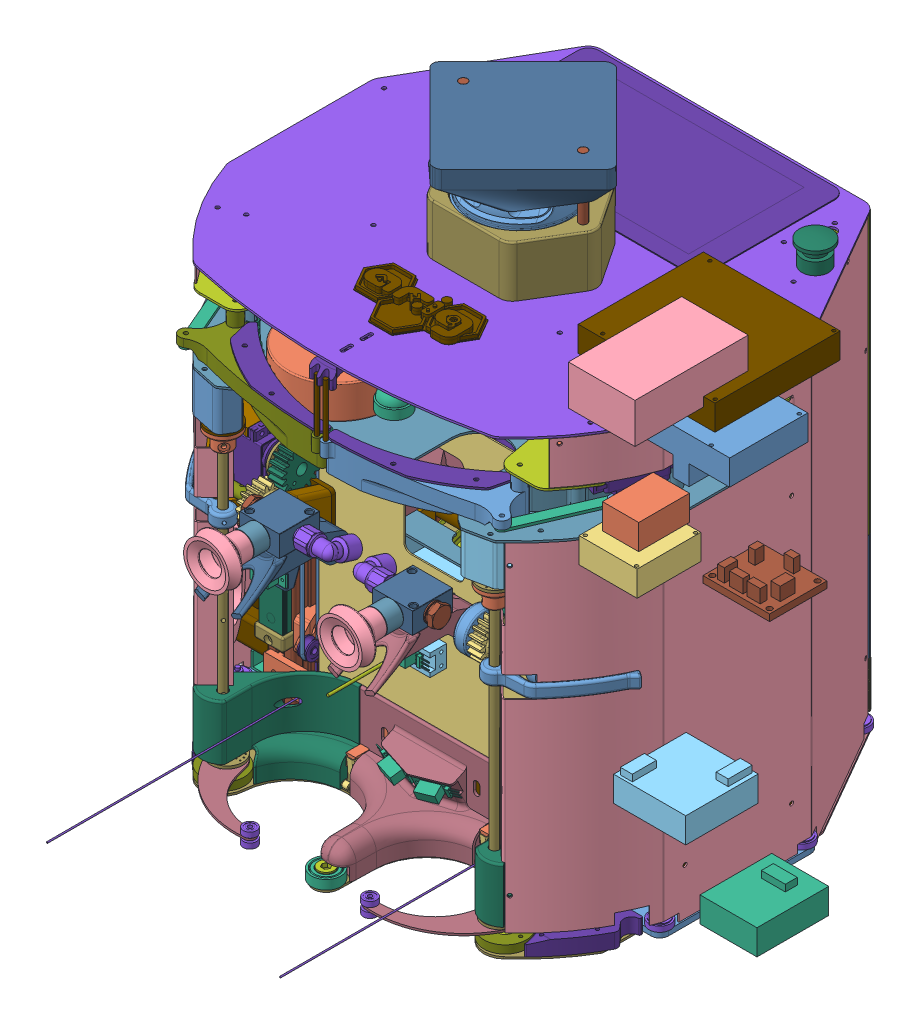
SolidWorks assembly 2019_Gros_robot, configuration Défaut. Lengths in mm. (continued)
Mates (geometry in assembly coordinates): (continued)
- Coaxiale36: concentric anti-aligned: cylinder of roulement-1 through (0 11.5 145.4518) axis (0 1 0) radius 4; cylinder of 20190123-2208-1 through (0 8.1 145.4518) axis (0 -1 0) radius 3.925
- Coïncidente121: coincident anti-aligned: plane of roulement-1 through (2.7957 15 140.7153) normal (0 1 0); plane of 20190123-2208-1 through (5.925 15 145.4518) normal (0 -1 0)
- Coaxiale37: concentric anti-aligned: cylinder of 20190208-2148-1 through (102 235.4 120.9526) axis (0 -1 0) radius 3; cylinder of 20190212-2200-1 through (102 57 120.9526) axis (0 1 0) radius 3.5
- Distance73: distance = 0.8 mm anti-aligned: plane of Roulement_d3xd10xe4-1 through (47.1943 17.95 156.201) normal (0 1 0); plane of 20190208-2207-1 through (102.5 18.75 117.5) normal (0 -1 0)
- Coaxiale39: concentric aligned: cylinder of Roulement_d3xd10xe4-1 through (45.0929 13.95 157.5553) axis (0 -1 0) radius 5; cylinder of 20190208-2207-1 through (45.0929 20.25 157.5553) axis (0 -1 0) radius 1.2
- Tangent1: tangent anti-aligned: cylinder of ? through (50 154.25 120) axis (0 -1 0) radius 38.1; cylinder of Roulement_d3xd10xe4-1 through (49.3866 13.95 163.0956) axis (0 -1 0) radius 5
- Coaxiale42: concentric aligned: cylinder of Roulement_d3xd10xe4-1 through (45.0929 13.95 157.5553) axis (0 -1 0) radius 5; cylinder of Roulement_d3xd10xe4-2 through (45.0929 21.05 157.5553) axis (0 -1 0) radius 5
- Distance74: distance = 0.8 mm anti-aligned: plane of Roulement_d3xd10xe4-2 through (42.6851 21.05 156.8828) normal (0 -1 0); plane of 20190208-2207-1 through (102.5 20.25 117.5) normal (0 1 0)
- Distance80: distance = 50 mm aligned: plane of Palet-1 through (-50 12.7 119.5978) normal (1 0 0); plane of assembly through (0 0 0) normal (1 0 0)
- Coïncidente140: coincident anti-aligned: plane of Robot2019_plaque bille porteuseAvant-1 through (0 7 0) normal (0 1 0); plane of 20190212-2200-1 through (-89.8589 7 116.7694) normal (0 -1 0)
- Coaxiale53: concentric: cylinder of Robot2019_plaque bille porteuseAvant-1 through (-50 7 120) axis (0 -1 0) radius 40; point of 20190212-2200-1
- Parallèle6: parallel anti-aligned: plane of Robot2017_BaseRoulante-1/Robot2015_BaseRoulante_piece01-1 through (0 11 60) normal (0 0 1); plane of 20190212-2200-1 through (-96 29 65) normal (0 0 -1)
- Coïncidente143: coincident anti-aligned: plane of microswitchGaletAss-1/microswitchGalet02-1 through (53.5 29 66) normal (1 0 0); plane of 20190212-2200-1 through (53.5 6.95 144) normal (-1 0 0)
- Coaxiale54: concentric anti-aligned: cylinder of microswitchGaletAss-1/microswitchGalet02-1 through (46.5 14.5 69) axis (1 0 0) radius 1; cylinder of 20190212-2200-1 through (68.5 14.5 69) axis (-1 0 0) radius 1.2
- Coaxiale55: concentric anti-aligned: cylinder of microswitchGaletAss-1/microswitchGalet02-1 through (46.5 23.5 69) axis (1 0 0) radius 1; cylinder of 20190212-2200-1 through (68.5 23.5 69) axis (-1 0 0) radius 1.2
- Coaxiale56: concentric aligned: cylinder of BillePorteuse2019-1 through (105.917 10 116.9526) axis (0 1 0) radius 6.4; cylinder of 20190214-0012-1 through (105.917 4.7 116.9526) axis (0 1 0) radius 8
- Coïncidente144: coincident anti-aligned: plane of BillePorteuse2019-1 through (110.9612 4.7 110.7432) normal (0 1 0); plane of 20190214-0012-1 through (105.917 4.7 116.9526) normal (0 -1 0)
- Coïncidente147: coincident anti-aligned: circle of Servo_HS-85-BB-1; circle of Access_HS-645_BrasRondPetitModele-1
- Coaxiale57: concentric anti-aligned: cylinder of 20190208-2207-1 through (102.5 20.25 117.5) axis (0 -1 0) radius 12; cylinder of Access_HS-645_BrasRondPetitModele-1 through (102.5 24.75 117.5) axis (0 1 0) radius 12
- Coïncidente148: coincident anti-aligned: plane of 20190208-2207-1 through (102.5 20.25 117.5) normal (0 1 0); plane of Access_HS-645_BrasRondPetitModele-1 through (100.0867 20.25 120.3703) normal (0 -1 0)
- Coaxiale58: concentric anti-aligned: cylinder of 20190208-2207-1 through (105.415 18.75 109.5155) axis (0 1 0) radius 1.2; cylinder of Access_HS-645_BrasRondPetitModele-1 through (105.415 30.25 109.5155) axis (0 -1 0) radius 0.5
- Coaxiale59: concentric aligned: cylinder of 20190208-2207-1 through (102.5 20.25 117.5) axis (0 -1 0) radius 12; cylinder of 20190208-2207-2 through (102.5 20.25 117.5) axis (0 -1 0) radius 12
- Angle2: planar angle = 3.185226 rad aligned: plane of 20190208-2207-1 through (102.5 18.75 117.5) normal (-0.572218 0 -0.820101); plane of 20190208-2207-2 through (102.5 18.75 117.5) normal (0.607446 0 0.794361)
- Distance82: distance = 96 mm anti-aligned: plane of Servo_HS-85-BB-1 through (96 25.85 124) normal (-1 0 0); plane of assembly through (0 0 0) normal (1 0 0)
- Distance83: distance = 117.5 mm: point of 20190208-2207-1; plane of assembly
- Distance84: distance = 30 mm aligned: plane of Servo_HS-85-BB-1 through (102.5 37 117.5) normal (0 1 0); plane of Robot2019_plaque bille porteuseAvant-1 through (0 7 0) normal (0 1 0)
- Coaxiale61: concentric aligned: cylinder of Robot2019_plaque bille porteuseAvant-1 through (105.917 7 116.9526) axis (0 -1 0) radius 16; cylinder of 20190214-0012-1 through (105.917 14.7 116.9526) axis (0 -1 0) radius 16
- Coïncidente151: coincident aligned: plane of 20190208-2207-1 through (102.5 20.25 117.5) normal (0 1 0); plane of 20190208-2207-2 through (102.5 20.25 117.5) normal (0 1 0)
- Coaxiale62: concentric aligned: cylinder of Robot2019_plaque bille porteuseAvant-1 through (100.1435 7 126.9526) axis (0 -1 0) radius 1.5; cylinder of 20190214-0012-1 through (100.1435 14.7 126.9526) axis (0 -1 0) radius 1.2
- Coaxiale63: concentric aligned: cylinder of 20181001-2148-1 through (-7.4687 58.1355 42.4725) axis (0.258819 -0.408218 0.875426) radius 0.65; cylinder of 20170416-2304-1/pololu gp2y0d805-1 through (3.2601 41.2137 78.7615) axis (0.258819 -0.408218 0.875426) radius 1
- Coïncidente152: coincident anti-aligned: plane of 20181001-2148-1 through (0 51.0665 85.3479) normal (0.258819 -0.408218 0.875426); plane of 20170416-2304-1/pololu gp2y0d805-1 through (1.0782 36.4945 78.234) normal (-0.258819 0.408218 -0.875426)
- Parallèle7: parallel aligned: plane of 20181001-2148-1 through (1.0353 36.8864 76.4144) normal (0 0.906308 0.422618); plane of 20170416-2304-1/pololu gp2y0d805-1 through (1.4924 43.9981 83.4383) normal (0 0.906308 0.422618)
- Coïncidente157: coincident anti-aligned: plane of Robot2019_plaque bille porteuseAvant-1 through (0 7 0) normal (0 1 0); plane of 20190219-0006-1 through (105.917 7 116.9526) normal (0 -1 0)
- Coaxiale64: concentric aligned: cylinder of Robot2019_plaque bille porteuseAvant-1 through (0 7 0) axis (0 -1 0) radius 173.7857; cylinder of 20190219-0006-1 through (0 18 0) axis (0 -1 0) radius 174
- Coïncidente158: coincident aligned: plane of 20190219-0006-1 through (0 7 0) normal (0 0 1); plane of assembly through (0 0 0) normal (0 0 1)
- Coïncidente159: coincident aligned: plane of Roulement_d3xd10xe4-1 through (47.1943 13.95 156.201) normal (0 -1 0); plane of Roulement_d3xd10xe4-3 through (160.2067 13.95 73.6245) normal (0 -1 0)
- Coaxiale65: concentric aligned: cylinder of 20190208-2207-2 through (158.1053 20.25 74.9788) axis (0 -1 0) radius 4; cylinder of Roulement_d3xd10xe4-3 through (158.1053 13.95 74.9788) axis (0 -1 0) radius 5
- Coïncidente161: coincident anti-aligned: plane of 20190219-0101-1 through (130 61.0678 59) normal (-1 0 0); plane of Robot2019_profiléX20_02-3 through (130 11 46.7) normal (1 0 0)
- Distance86: distance = 1 mm aligned: plane of 20190219-0101-1 through (130 61.0678 59) normal (0 0 1); plane of Robot2019_profiléX20_02-3 through (123.3 11 60) normal (0 0 1)
- Coïncidente162: coincident aligned: plane of 20190219-0101-1 through (163 14.6933 37) normal (1 0 0); plane of 20190219-0101-2 through (163 87.4423 -37) normal (1 0 0)
- Coïncidente163: coincident aligned: plane of 20190219-0101-1 through (130 61.0678 50) normal (0 1 0); plane of 20190219-0101-2 through (130 61.0678 -50) normal (0 1 0)
- Distance87: distance = 1 mm aligned: plane of 20190219-0101-2 through (130 41.0678 -59) normal (0 0 -1); plane of Robot2019_profiléX20_02-4 through (128 11 -60) normal (0 0 -1)
- Coaxiale66: concentric aligned: cylinder of 20190208-2148-1 through (102 235.4 120.9526) axis (0 -1 0) radius 3; cylinder of 20190220-2148-1 through (102 186.4 120.9526) axis (0 -1 0) radius 3.1
- Coaxiale67: concentric aligned: cylinder of Servo_HS-85-BB-2 through (102 241.9 120.9526) axis (0 1 0) radius 2.75; cylinder of Access_HS-645_BrasRondPetitModele-2 through (102 244.9 120.9526) axis (0 1 0) radius 2.75
- Coïncidente164: coincident anti-aligned: plane of Servo_HS-85-BB-2 through (102 241.9 120.9526) normal (0 -1 0); plane of Access_HS-645_BrasRondPetitModele-2 through (99.4128 241.9 121.8847) normal (0 1 0)
- Coïncidente165: coincident anti-aligned: plane of Robot2019_plaque du dessus-1 through (0 276 -355) normal (0 -1 0); plane of Servo_HS-85-BB-2 through (102 276 120.9526) normal (0 1 0)
- Coaxiale68: concentric anti-aligned: cylinder of 20190208-2148-1 through (102 235.4 120.9526) axis (0 -1 0) radius 3; cylinder of Access_HS-645_BrasRondPetitModele-2 through (102 244.9 120.9526) axis (0 1 0) radius 12
- Coaxiale70: concentric aligned: cylinder of Access_HS-645_BrasRondPetitModele-2 through (102 244.9 120.9526) axis (0 1 0) radius 12; cylinder of 20190221-0033-1 through (102 240.4 120.9526) axis (0 1 0) radius 12
- Coïncidente168: coincident anti-aligned: plane of Access_HS-645_BrasRondPetitModele-2 through (98.472 240.4 122.2237) normal (0 -1 0); plane of 20190221-0033-1 through (99.4389 240.4 117.88) normal (0 1 0)
- Coaxiale71: concentric anti-aligned: cylinder of Access_HS-645_BrasRondPetitModele-2 through (95.5972 250.4 113.2712) axis (0 -1 0) radius 0.5; cylinder of 20190221-0033-1 through (95.5972 225.4 113.2712) axis (0 1 0) radius 1.2
- Distance91: distance = 4 mm aligned: plane of Raspberry pi3 Screen assembly-1 through (-9.296 346 -101.85) normal (0 1 0); plane of assembly through (0 350 0) normal (0 1 0)
- Coaxiale72: concentric aligned: cylinder of 20190208-2148-1 through (99.6956 229.4 122.8734) axis (0.768138 0 -0.640285) radius 1.25; cylinder of 20190221-0033-1 through (92.7823 229.4 128.636) axis (0.768138 0 -0.640285) radius 1.5
- Coaxiale73: concentric aligned: cylinder of 20190208-2148-1 through (99.6956 181.4 122.8734) axis (0.768138 0 -0.640285) radius 1.25; cylinder of 20190220-2148-1 through (108.1451 181.4 115.8303) axis (0.768138 0 -0.640285) radius 1.2
- AngleLimite1: limit planar angle = 0.418879 rad aligned: plane of 20190220-2148-1 through (102 181.4 120.9526) normal (0.913545 0 0.406737); plane of assembly through (0 0 0) normal (1 0 0)
- Coïncidente169: coincident aligned: plane of Carter2019-1 through (0 7 0) normal (0 0 1); plane of assembly through (0 0 0) normal (0 0 1)
- Coïncidente170: coincident aligned: plane of Carter2019-1 through (0 7 0) normal (1 0 0); plane of assembly through (0 0 0) normal (1 0 0)
- Coïncidente171: coincident anti-aligned: plane of Robot2017_BaseRoulante-1/Robot2015_BaseRoulante_piece01-1 through (0 7 0) normal (0 -1 0); plane of Carter2019-1 through (0 7 0) normal (0 1 0)
- Coïncidente172: coincident anti-aligned: plane of Robot2019_plaque du dessus-1 through (0 276 -355) normal (0 -1 0); plane of 20190223-1730-1 through (-0.1299 276 -354.8724) normal (0 1 0)
- Coïncidente173: coincident anti-aligned: plane of Servo_HS-85-BB-2 through (124.7356 246 115.3317) normal (0.5 0 0.866025); plane of 20190223-1730-1 through (125.0387 276 115.1567) normal (-0.5 0 -0.866025)
- Coaxiale75: concentric aligned: cylinder of Servo_HS-85-BB-2 through (93.6429 257.15 125.7776) axis (0 -1 0) radius 1.5; cylinder of 20190223-1730-1 through (93.6429 276 125.7776) axis (0 -1 0) radius 1.2
- Parallèle9: parallel aligned: plane of assembly through (0 0 0) normal (1 0 0); plane of 20190223-1730-1 through (-0.1299 256 0.1276) normal (1 0 0)
- Coaxiale76: concentric aligned: cylinder of 20181002-0030-1/20181002-0031-4 through (0 293.5 0) axis (0 -1 0) radius 141; cylinder of 20181002-0216-1/20181002-0217-1 through (0 296.5 0) axis (0 -1 0) radius 141
- Coïncidente175: coincident anti-aligned: plane of 20181001-2148-1 through (0 51.0665 85.3479) normal (-0.258819 -0.408218 0.875426); plane of 20170416-2304-2/pololu gp2y0d805-1 through (-1.0782 44.6512 82.0376) normal (0.258819 0.408218 -0.875426)
- Coaxiale77: concentric aligned: cylinder of 20181001-2148-1 through (7.4687 58.1355 42.4725) axis (-0.258819 -0.408218 0.875426) radius 0.65; cylinder of 20170416-2304-2/pololu gp2y0d805-1 through (-3.2601 41.2137 78.7615) axis (-0.258819 -0.408218 0.875426) radius 1
- Parallèle10: parallel aligned: plane of 20181001-2148-1 through (1.0353 36.8864 76.4144) normal (0 0.906308 0.422618); plane of 20170416-2304-2/pololu gp2y0d805-1 through (-1.4924 43.9981 83.4383) normal (0 0.906308 0.422618)
- Coaxiale78: concentric aligned: cylinder of Robot2019_plaque du dessus-1 through (0 267.5 0) axis (0 1 0) radius 27; cylinder of 20190221-0152-1 through (0 274.2 0) axis (0 1 0) radius 25.3
- Distance94: distance = 1.5 mm anti-aligned: plane of 20190221-0152-1 through (0 311 0) normal (0 -1 0); plane of 20181002-0030-1/20181002-0031-2 through (0 309.5 0) normal (0 1 0)
- Coïncidente177: coincident anti-aligned: plane of 20190221-0152-1; plane of assembly through (0 0 0) normal (1 0 0)
- Coïncidente178: coincident anti-aligned: plane of Symétrie20181002-0216-3/Symétrie20181002-0217-1 through (114.2513 290.5 136.5049) normal (0 -1 0); plane of 20190225-2214-1 through (118.6064 290.5 132.1497) normal (0 1 0)
- Coaxiale79: concentric aligned: cylinder of Symétrie20181002-0216-3/Symétrie20181002-0217-1 through (118.6064 430.1481 132.1497) axis (0 -1 0) radius 1.5; cylinder of 20190225-2214-1 through (118.6064 290.5 132.1497) axis (0 -1 0) radius 1.5
- Coaxiale80: concentric anti-aligned: cylinder of Access_HS-485_BrasReglablePartieB-1 through (143.565 290.05 74.3045) axis (0 1 0) radius 0.5; cylinder of 20190225-2214-1 through (143.565 290.5 74.3045) axis (0 -1 0) radius 1.5
- Coïncidente179: coincident anti-aligned: plane of 20181002-0030-1/20181002-0031-2 through (0 309.5 0) normal (0 1 0); plane of Robot2019_plaque elec-1 through (0 309.5 -355) normal (0 -1 0)
- Coaxiale83: concentric anti-aligned: cylinder of Robot2019_plaque elec-1 through (143 301 86.913) axis (0 1 0) radius 1.5; cylinder of Servo_HS-485-HB-1 through (143 309.5 86.913) axis (0 -1 0) radius 1.5
- Parallèle13: parallel aligned: plane of Servo_HS-485-HB-1 through (159.9911 312.35 48.1691) normal (0.95652 0 0.291667); plane of Robot2019_plaque elec-1 through (141.4855 301 40.4511) normal (0.95652 0 0.291667)
- AngleLimite2: limit planar angle = 0 rad anti-aligned: plane of Robot2019_plaque du dessus-1 through (30 275.999 141.0123) normal (0.130526 0 0.991445); plane of Symétrie20181002-0216-3/Symétrie20181002-0217-1 through (0.3812 243.6998 144.987) normal (-0.130526 0 -0.991445)
- Distance95: distance = 5 mm aligned: plane of Robot2019_plaque superieure-2 through (0 345 -355) normal (0 1 0); plane of assembly through (0 350 0) normal (0 1 0)
- Coïncidente185: coincident anti-aligned: plane of rplidar-a2-1 through (0 362.5 0) normal (0 -1 0); plane of 20161105-0900-1 through (0 362.5 0) normal (0 1 0)
- Coaxiale85: concentric anti-aligned: cylinder of rplidar-a2-1 through (-20.8597 362.5 20.8597) axis (0 1 0) radius 1.6; cylinder of 20161105-0900-1 through (-20.8597 380.5 20.8597) axis (0 -1 0) radius 1.5
- Coaxiale86: concentric anti-aligned: cylinder of rplidar-a2-1 through (-20.8597 362.5 -20.8597) axis (0 1 0) radius 1.6; cylinder of 20161105-0900-1 through (-20.8597 380.5 -20.8597) axis (0 -1 0) radius 1.5
- Coaxiale87: concentric aligned: cylinder of 20161105-0900-1 through (-45 380.5 -2.5) axis (0 -1 0) radius 3; cylinder of 20161106-1538-1 through (-45 430 -2.5) axis (0 -1 0) radius 3
- Coaxiale88: concentric aligned: cylinder of 20190313-2117-1 through (-45 430 -2.5) axis (0 -1 0) radius 3.1; cylinder of 20161106-1538-1 through (-45 430 -2.5) axis (0 -1 0) radius 3
- Coaxiale89: concentric aligned: cylinder of 20161105-0900-1 through (45 380.5 -2.5) axis (0 -1 0) radius 3; cylinder of 20161106-1538-2 through (45 430 -2.5) axis (0 -1 0) radius 3
- Coaxiale90: concentric aligned: cylinder of 20190313-2117-1 through (45 430 -2.5) axis (0 -1 0) radius 3.1; cylinder of 20161106-1538-2 through (45 430 -2.5) axis (0 -1 0) radius 3
- Coïncidente186: coincident aligned: plane of 20190313-2117-1 through (0 430 -2.5) normal (0 1 0); plane of 20161106-1538-2 through (45 430 -2.5) normal (0 1 0)
- Coïncidente187: coincident aligned: plane of 20190313-2117-1 through (0 430 -2.5) normal (0 1 0); plane of 20161106-1538-1 through (-45 430 -2.5) normal (0 1 0)
- Coïncidente188: coincident anti-aligned: plane of Robot2019_plaque superieure-2 through (0 345 -355) normal (0 1 0); plane of 20161105-0900-1 through (45 345 -2.5) normal (0 -1 0)
- Coïncidente189: coincident aligned: plane of 20190313-2117-1 through (0 430 -2.5) normal (0 1 0); plane of assembly through (0 430 0) normal (0 1 0)
- Coïncidente190: coincident aligned: plane of 20161105-0900-1 through (0 345 0) normal (0 0 1); plane of assembly through (0 0 0) normal (0 0 1)
- Coïncidente191: coincident aligned: plane of 20161105-0900-1 through (0 345 0) normal (1 0 0); plane of assembly through (0 0 0) normal (1 0 0)
- Distance96: distance = 1 mm anti-aligned: plane of Robot2019_plaque superieure-2 through (76.184 342 -152) normal (-1 0 0); plane of Raspberry pi3 Screen assembly-1 through (75.184 340.04 -50) normal (1 0 0)
- Distance97: distance = 2 mm aligned: plane of 20170416-2304-3/SupportCapteurPololu-1 through (-128 238.5 -30) normal (-1 0 0); plane of Robot2019_profiléX20_02-2 through (-130 11 -46.7) normal (-1 0 0)
- Distance98: distance = 40 mm aligned: plane of 20170416-2304-3/SupportCapteurPololu-1 through (-120 226 0) normal (0 0 1); plane of Robot2019_profiléX20_02-2 through (-128 11 -40) normal (0 0 1)
- Distance99: distance = 50 mm aligned: plane of 20170416-2304-3/SupportCapteurPololu-1 through (-128 226 -30) normal (0 -1 0); plane of Robot2019_plaque du dessus-1 through (0 276 -355) normal (0 -1 0)
- Distance100: distance = 3 mm anti-aligned: plane of Adafruit_TCS34725-1 through (-106.6 273 31) normal (0 1 0); plane of Robot2019_plaque du dessus-1 through (0 276 -355) normal (0 -1 0)
- Distance102: distance = 9 mm anti-aligned: plane of Adafruit_TCS34725-1 through (-106.6 269 31) normal (0 0 1); plane of Robot2019_profiléX20_02-1 through (-123.3 11 40) normal (0 0 -1)
- Distance103: distance = 3 mm aligned: plane of Robot2019_profiléX20_02-1 through (-130 11 42) normal (-1 0 0); plane of Adafruit_TCS34725-1 through (-127 269 31) normal (-1 0 0)
- Coïncidente199: coincident anti-aligned: plane of Robot2019_profiléX20_02-1 through (-123.3 11 40) normal (0 0 -1); plane of 20190227-2336-1 through (-122.35 269 40) normal (0 0 1)
- Distance104: distance = 1.5 mm aligned: plane of 20190227-2336-1 through (-128.5 269 37) normal (-1 0 0); plane of Robot2019_profiléX20_02-1 through (-130 11 42) normal (-1 0 0)
- Coïncidente201: coincident anti-aligned: plane of Adafruit_TCS34725-1 through (-106.6 269 31) normal (0 -1 0); plane of 20190227-2336-1 through (-120 269 40) normal (0 1 0)
- Coïncidente205: coincident anti-aligned: plane of Robot2019_profiléX20_02-1 through (-112 11 40) normal (0 0 -1); plane of 20190228-0009-1 through (-147.0576 165.5788 40) normal (0 0 1)
- Coïncidente206: coincident anti-aligned: plane of 20190228-0009-1 through (0 165.5788 39.25) normal (-1 0 0); plane of assembly through (0 0 0) normal (1 0 0)
- Coïncidente207: coincident anti-aligned: plane of 20181005-1508-1/20181006-0057-1 through (-48 165.5788 10.194) normal (0 -1 0); plane of 20190228-0009-1 through (-127.5 165.5788 49) normal (0 1 0)
- Coïncidente208: coincident anti-aligned: plane of 20181005-1508-1/Servo_HS-485-HB-1 through (-34 207.5 -31.6025) normal (1 0 0); plane of Robot2015_supportServo02-1 through (-34 217.5 -3.6025) normal (-1 0 0)
- Coaxiale91: concentric aligned: cylinder of 20181005-1508-1/20181006-0057-1 through (-39 241.5 -36.6025) axis (-1 0 0) radius 1.2; cylinder of Robot2015_supportServo02-1 through (-32.5 241.5 -36.6025) axis (-1 0 0) radius 1.5
- Coaxiale92: concentric aligned: cylinder of 20181005-1508-1/20181006-0057-1 through (-39 241.5 -26.6025) axis (-1 0 0) radius 1.2; cylinder of Robot2015_supportServo02-1 through (-32.5 241.5 -26.6025) axis (-1 0 0) radius 1.5
- Coïncidente209: coincident aligned: plane of Robot2019_plaque superieure-2 through (0 343.5 0) normal (0 0 1); plane of assembly through (0 0 0) normal (0 0 1)
- Coïncidente210: coincident aligned: plane of Robot2019_plaque superieure-2 through (0 343.5 0) normal (1 0 0); plane of assembly through (0 0 0) normal (1 0 0)
- Coaxiale93: concentric anti-aligned: cylinder of APEM_A01ES_A0154B-1 through (121.8383 364 -100) axis (0 -1 0) radius 8; cylinder of Robot2019_plaque superieure-2 through (121.8383 342 -100) axis (0 1 0) radius 8
- Coïncidente211: coincident anti-aligned: plane of APEM_A01ES_A0154B-1 through (126.8383 345 -91.3397) normal (0 -1 0); plane of Robot2019_plaque superieure-2 through (0 345 -355) normal (0 1 0)
- Coïncidente212: coincident anti-aligned: plane of Raspberry pi3 Screen assembly-1 through (-7.916 340.04 -100.3) normal (0 -1 0); plane of 20190301-2106-1 through (47.184 340.04 -143.825) normal (0 1 0)
- Coaxiale94: concentric anti-aligned: cylinder of Raspberry pi3 Screen assembly-1 through (55.184 340.04 -135.65) axis (0 -1 0) radius 1.5; cylinder of 20190301-2106-1 through (55.184 335.04 -135.65) axis (0 1 0) radius 1.5
- Parallèle14: parallel aligned: plane of Raspberry pi3 Screen assembly-1 through (75.184 340.04 -150.6) normal (0 0 -1); plane of 20190301-2106-1 through (47.184 337.04 -143.825) normal (0 0 -1)
- Coïncidente214: coincident anti-aligned: plane of Robot2019_plaque superieure-2 through (0 343.5 -355) normal (0 -1 0); plane of 20190301-2139-1 through (0 343.5 115) normal (0 1 0)
- Coïncidente215: coincident aligned: plane of 20190301-2139-1 through (0 343.5 0) normal (1 0 0); plane of assembly through (0 0 0) normal (1 0 0)
- Coïncidente216: coincident aligned: plane of 20190301-2139-1 through (0 343.5 0) normal (0 0 1); plane of assembly through (0 0 0) normal (0 0 1)
- Coïncidente217: coincident aligned: plane of Robot2019_plaque elec-1 through (0 309.5 0) normal (0 0 1); plane of assembly through (0 0 0) normal (0 0 1)
- Coïncidente218: coincident aligned: plane of Robot2019_plaque elec-1 through (0 309.5 0) normal (1 0 0); plane of assembly through (0 0 0) normal (1 0 0)
- Coïncidente219: coincident aligned: plane of Robot2019_plaque du dessus-1 through (0 276 0) normal (0 0 1); plane of assembly through (0 0 0) normal (0 0 1)
- Coaxiale95: concentric anti-aligned: cylinder of Robot2019_plaque superieure-2 through (30 343.5 80) axis (0 1 0) radius 1.5; cylinder of LogoARIG2-1 through (30 353.3941 80) axis (0 -1 0) radius 1.2
- Coaxiale96: concentric anti-aligned: cylinder of Robot2019_plaque superieure-2 through (-30 343.5 80) axis (0 1 0) radius 1.5; cylinder of LogoARIG2-1 through (-30 353.3941 80) axis (0 -1 0) radius 1.2
- Coïncidente220: coincident anti-aligned: plane of Robot2019_plaque superieure-2 through (0 345 -355) normal (0 1 0); plane of LogoARIG2-1 through (-42.5 345 104) normal (0 -1 0)
- Coaxiale99: concentric aligned: cylinder of Robot2019_plaque du dessus-1 through (56.5 275.999 -145) axis (0 1 0) radius 1.25; cylinder of GP2D-2 through (56.5 277.5 -145) axis (0 1 0) radius 1.6
- Coaxiale100: concentric aligned: cylinder of Robot2019_plaque du dessus-1 through (93.5 275.999 -145) axis (0 1 0) radius 1.25; cylinder of GP2D-2 through (93.5 277.5 -145) axis (0 1 0) radius 1.6
- Coïncidente223: coincident anti-aligned: plane of Raspberry pi3 Screen assembly-1 through (-91.016 340.04 -50) normal (0 0 1); plane of Robot2019_plaque superieure-2 through (5.7325 342 -50) normal (0 0 -1)
- Coïncidente224: coincident anti-aligned: plane of 20181006-0254-1 through (-106.5 343.5 -156.0025) normal (0 1 0); plane of Robot2019_plaque superieure-2 through (0 343.5 -355) normal (0 -1 0)
- Coaxiale101: concentric anti-aligned: cylinder of Raspberry pi3 Screen assembly-1 through (-71.016 340.04 -135.65) axis (0 -1 0) radius 1.5; cylinder of 20190301-2106-2 through (-71.016 335.04 -135.65) axis (0 1 0) radius 1.5
- Coaxiale102: concentric anti-aligned: cylinder of Raspberry pi3 Screen assembly-1 through (-71.016 340.04 -70) axis (0 -1 0) radius 1.5; cylinder of 20190301-2106-2 through (-71.016 335.04 -70) axis (0 1 0) radius 1.5
- Coïncidente225: coincident anti-aligned: plane of Raspberry pi3 Screen assembly-1 through (-7.916 340.04 -100.3) normal (0 -1 0); plane of 20190301-2106-2 through (-63.016 340.04 -61.825) normal (0 1 0)
- Coaxiale103: concentric anti-aligned: cylinder of 20181006-0254-1 through (-30 268.5 -156.0025) axis (0 0 -1) radius 1.5; cylinder of LogoARIG2-2 through (-30 268.5 -168.3967) axis (0 0 1) radius 1.2
- Coaxiale104: concentric anti-aligned: cylinder of 20181006-0254-1 through (30 268.5 -156.0025) axis (0 0 -1) radius 1.5; cylinder of LogoARIG2-2 through (30 268.5 -168.3967) axis (0 0 1) radius 1.2
- Coïncidente226: coincident anti-aligned: plane of 20181006-0254-1 through (0 343.5 -160.0025) normal (0 0 -1); plane of LogoARIG2-2 through (42.5 244.5 -160.0025) normal (0 0 1)
- Coïncidente227: coincident anti-aligned: plane of Robot2019_plaque superieure-2 through (0 343.5 -355) normal (0 -1 0); plane of 20190308-1510-1 through (0 343.5 0) normal (0 1 0)
- Coïncidente228: coincident aligned: plane of 20190308-1510-1 through (0 336.5 0) normal (0 0 1); plane of assembly through (0 0 0) normal (0 0 1)
- Coïncidente229: coincident aligned: plane of 20190308-1510-1 through (0 336.5 0) normal (1 0 0); plane of assembly through (0 0 0) normal (1 0 0)
- Coïncidente232: coincident anti-aligned: plane of Robot2019_plaque superieure-2 through (0 343.5 -355) normal (0 -1 0); plane of 20190308-2149-1 through (0 343.5 0) normal (0 1 0)
- Coaxiale105: concentric anti-aligned: cylinder of Robot2019_plaque superieure-2 through (-155 342 -53) axis (0 1 0) radius 1.5; cylinder of 20190308-2149-1 through (-155 354.8137 -53) axis (0 -1 0) radius 1.2
- Coaxiale106: concentric anti-aligned: cylinder of Robot2019_plaque superieure-2 through (-140 342 87) axis (0 1 0) radius 1.5; cylinder of 20190308-2149-1 through (-140 354.8137 87) axis (0 -1 0) radius 1.2
- Coïncidente233: coincident anti-aligned: line of 20190308-1510-1 through (152.4215 312 -59.2282) axis (-0.5 0 -0.866025); line of interrupteur principal-1 through (137.9215 312 -84.3429) axis (0.5 0 0.866025)
- Coïncidente234: coincident anti-aligned: line of 20190308-1510-1 through (137.9215 312 -84.3429) axis (0 1 0); line of interrupteur principal-1 through (137.9215 334 -84.3429) axis (0 -1 0)
- Coïncidente235: coincident anti-aligned: plane of Robot2019_plaque elec-1 through (0 311 -355) normal (0 1 0); plane of 20190309-0049-1 through (-60 311 83) normal (0 -1 0)
- Coaxiale107: concentric anti-aligned: cylinder of Robot2019_plaque elec-1 through (-70 309.5 40) axis (0 1 0) radius 1.5; cylinder of 20190309-0049-1 through (-70 354.3137 40) axis (0 -1 0) radius 1.2
- Coaxiale108: concentric anti-aligned: cylinder of Robot2019_plaque elec-1 through (70 309.5 40) axis (0 1 0) radius 1.5; cylinder of 20190309-0049-1 through (70 354.3137 40) axis (0 -1 0) radius 1.2
- Coïncidente236: coincident anti-aligned: plane of Robot2019_profiléX20_02-1 through (-130 11 53.3) normal (-1 0 0); plane of 20190309-0127_Corniere_15.5x27.5x1.5-1 through (-130 260.5 59) normal (1 0 0)
- Distance106: distance = 1 mm aligned: plane of Robot2019_profiléX20_02-1 through (-128 11 60) normal (0 0 1); plane of 20190309-0127_Corniere_15.5x27.5x1.5-1 through (-130 276 59) normal (0 0 1)
- Coïncidente238: coincident anti-aligned: plane of Robot2019_plaque du dessus-1 through (0 276 -355) normal (0 -1 0); plane of 20190309-0127_Corniere_15.5x27.5x1.5-1 through (-130 276 59) normal (0 1 0)
- Coïncidente242: coincident anti-aligned: plane of 20181006-0254-1 through (0 343.5 -156.0025) normal (0 0 1); plane of Ventilo-2 through (75 318.5 -156.0025) normal (0 0 -1)
- Coaxiale109: concentric aligned: cylinder of 20181006-0254-1 through (91 302.5 -156.0025) axis (0 0 -1) radius 1.5; cylinder of Ventilo-2 through (91 302.5 -146.0025) axis (0 0 -1) radius 1.5
- Coaxiale110: concentric aligned: cylinder of 20181006-0254-1 through (59 334.5 -156.0025) axis (0 0 -1) radius 1.5; cylinder of Ventilo-2 through (59 334.5 -146.0025) axis (0 0 -1) radius 1.5
- Distance107: distance = 10 mm aligned: plane of GP2D-2 through (56.5 287.5 -145) normal (0 1 0); plane of Robot2019_plaque du dessus-1 through (0 277.5 -355) normal (0 1 0)
- Coïncidente245: coincident anti-aligned: plane of TelemetreTOF_RB-Mce-01-1 through (-74.5065 272.4886 -143) normal (-0.139173 0.990268 0); plane of 20190314-1109-1 through (-74.5065 272.4886 -143) normal (0.139173 -0.990268 0)
- Coaxiale111: concentric anti-aligned: cylinder of TelemetreTOF_RB-Mce-01-1 through (-74.2977 271.0032 -133) axis (-0.139173 0.990268 0) radius 1; cylinder of 20190314-1109-1 through (-75.8982 282.3912 -133) axis (0.139173 -0.990268 0) radius 1.5
- Coaxiale112: concentric anti-aligned: cylinder of TelemetreTOF_RB-Mce-01-1 through (-74.2977 271.0032 -153) axis (-0.139173 0.990268 0) radius 1; cylinder of 20190314-1109-1 through (-75.8982 282.3912 -153) axis (0.139173 -0.990268 0) radius 1.5
- Coïncidente246: coincident anti-aligned: plane of Robot2019_plaque du dessus-1 through (0 276 -355) normal (0 -1 0); plane of 20190314-1109-1 through (-84.0884 276 -143) normal (0 1 0)
- Coaxiale113: concentric: cylinder of Robot2019_plaque du dessus-1 through (-75 276 -133) axis (0 1 0) radius 1.5; point of 20190314-1109-1
- Parallèle15: parallel aligned: plane of 20181006-0254-1 through (0 343.5 -160.0025) normal (0 0 -1); plane of 20190314-1109-1 through (-84.8106 281.1387 -155.5) normal (0 0 -1)
- Coïncidente247: coincident anti-aligned: plane of 20181005-1508-1/20181005-2259-1 through (50 7 -156.0025) normal (0 0 -1); plane of 20181006-0254-1 through (0 343.5 -156.0025) normal (0 0 1)
- Coïncidente248: coincident anti-aligned: plane of 20181005-1508-1/20181005-2259-1 through (-50 7 -156.0025) normal (0 0 -1); plane of 20181006-0255-1 through (0 133.2 -156.0025) normal (0 0 1)
- Coaxiale114: concentric aligned: cylinder of 20181006-0254-1 through (-100.4378 343.5 -153.5025) axis (0 1 0) radius 6.5; cylinder of 20181006-0255-1 through (-100.4378 133.2 -153.5025) axis (0 1 0) radius 6.5
- Coaxiale115: concentric aligned: cylinder of 20181005-1508-1/20181005-2259-1 through (0 93.2 -141.0025) axis (0 0 -1) radius 1.2; cylinder of 20181006-0255-1 through (0 93.2 -156.0025) axis (0 0 -1) radius 1.5
- Coïncidente249: coincident anti-aligned: plane of 20181006-0255-1 through (10.5 53.2 -156.5025) normal (0 0 1); plane of Palet-2 through (51.9 38.1 -156.5025) normal (0 0 -1)
- Distance108: distance = 50 mm anti-aligned: plane of Palet-2 through (50 38.1 -143.8025) normal (-1 0 0); plane of assembly through (0 0 0) normal (1 0 0)
- Tangent2: tangent anti-aligned: cylinder of Palet-2 through (51.9 38.1 -156.5025) axis (0 0 1) radius 38.1; plane of assembly through (0 0 0) normal (0 1 0)
- Tangent3: tangent anti-aligned: plane of 20181005-1508-1/20181005-2259-1 through (90 156.9313 499843.9975) normal (-1 0 0); cylinder of Palet-2 through (51.9 38.1 -156.5025) axis (0 0 1) radius 38.1
- Coaxiale116: concentric anti-aligned: cylinder of TelemetreTOF_RB-Mce-01-2 through (97.5 42 66) axis (0 0 -1) radius 1; cylinder of 20190331-1440-1 through (97.5 42 60) axis (0 0 1) radius 1.5
- Coaxiale117: concentric anti-aligned: cylinder of TelemetreTOF_RB-Mce-01-2 through (77.5 42 66) axis (0 0 -1) radius 1; cylinder of 20190331-1440-1 through (77.5 42 60) axis (0 0 1) radius 1.5
- Coïncidente250: coincident anti-aligned: plane of TelemetreTOF_RB-Mce-01-2 through (87.5 42 64.5) normal (0 0 -1); plane of 20190331-1440-1 through (87.5 42 64.5) normal (0 0 1)
- Coïncidente251: coincident anti-aligned: plane of Robot2019_profiléX20_02-3 through (112 11 60) normal (0 0 1); plane of 20190331-1440-1 through (87.5 42 60) normal (0 0 -1)
- Distance109: distance = 2 mm aligned: plane of 20190331-1440-1 through (128 31 97.7002) normal (1 0 0); plane of Robot2019_profiléX20_02-3 through (130 11 58) normal (1 0 0)
- Distance110: distance = 20 mm anti-aligned: plane of 20190331-1440-1 through (102.5 31 60) normal (0 -1 0); plane of Robot2017_BaseRoulante-1/Robot2015_BaseRoulante_piece01-1 through (0 11 0) normal (0 1 0)
- Coïncidente254: coincident anti-aligned: plane of 20161105-0900-1 through (0 380.5 0) normal (0 1 0); plane of 20190331-1545-1 through (0 380.5 0) normal (0 -1 0)
- Coaxiale118: concentric anti-aligned: cylinder of 20161106-1538-1 through (-45 430 -2.5) axis (0 -1 0) radius 3; cylinder of 20190331-1545-1 through (-45 380.5 -2.5) axis (0 1 0) radius 3
- Coaxiale119: concentric anti-aligned: cylinder of 20161106-1538-2 through (45 430 -2.5) axis (0 -1 0) radius 3; cylinder of 20190331-1545-1 through (45 380.5 -2.5) axis (0 1 0) radius 3
- Coaxiale120: concentric anti-aligned: cylinder of 20180929-0119-1/12v-silent-dc-motor-146rpm-encoder-desc-dime-1 through (-9.8995 248.4645 12.6005) axis (0 1 0) radius 1.25; cylinder of 20190331-1640-1 through (-9.8995 260 12.6005) axis (0 -1 0) radius 1.5
- Coaxiale121: concentric anti-aligned: cylinder of 20180929-0119-1/12v-silent-dc-motor-146rpm-encoder-desc-dime-1 through (-9.8995 248.4645 32.3995) axis (0 1 0) radius 1.25; cylinder of 20190331-1640-1 through (-9.8995 260 32.3995) axis (0 -1 0) radius 1.5
- Coïncidente255: coincident anti-aligned: plane of 20180929-0119-1/12v-silent-dc-motor-146rpm-encoder-desc-dime-1 through (12.7279 257 9.7721) normal (0 1 0); plane of 20190331-1640-1 through (0 257 22.5) normal (0 -1 0)
- Parallèle18: parallel aligned: plane of 20181005-1508-1/20181006-0057-1 through (-48 251 27.3975) normal (0 0 1); plane of 20190331-1640-1 through (-45 222 45.5) normal (0 0 1)
- Coaxiale122: concentric aligned: cylinder of 20190309-0127_Corniere_15.5x27.5x1.5-1 through (-145.7716 272 28.3351) axis (0 1 0) radius 1.5; cylinder of 20190309-0128-1 through (-145.7716 260.5 28.3351) axis (0 1 0) radius 1.5
- Coaxiale123: concentric aligned: cylinder of 20190309-0127_Corniere_15.5x27.5x1.5-1 through (-134 267 50) axis (1 0 0) radius 2.5; cylinder of 20190309-0128-1 through (-157.5 267 50) axis (1 0 0) radius 5
- Coaxiale124: concentric aligned: cylinder of 20170416-2304-3/pololu gp2y0d805-1 through (-120 235.9 -3) axis (0 1 0) radius 1; cylinder of SupportCapteurPololuSpecial2019-1 through (-120 226 -3) axis (0 1 0) radius 0.75
- Parallèle19: parallel aligned: plane of 20170416-2304-3/pololu gp2y0d805-1 through (-115.5 238.4 -0.5) normal (0 0 1); plane of SupportCapteurPololuSpecial2019-1 through (-120 226 0) normal (0 0 1)
- Coïncidente257: coincident anti-aligned: plane of 20170416-2304-3/pololu gp2y0d805-1 through (-115.5 236.8 -0.5) normal (0 -1 0); plane of SupportCapteurPololuSpecial2019-1 through (-120 236.8 -15) normal (0 1 0)
- Coïncidente258: coincident anti-aligned: plane of Robot2017_BaseRoulante-1/Robot2015_profiléX20_01-1 through (-46 176 -60) normal (0 0 -1); plane of Robot2015_BaseRoulante_piece15-1 through (95 119.5 -60) normal (0 0 1)
- Distance111: distance = 70 mm aligned: plane of Robot2015_BaseRoulante_piece15-1 through (95 81 -60) normal (0 1 0); plane of Robot2017_BaseRoulante-1/Robot2015_BaseRoulante_piece01-1 through (0 11 0) normal (0 1 0)
- Distance112: distance = 95 mm anti-aligned: plane of Robot2015_BaseRoulante_piece15-1 through (-95 79.5 -60) normal (-1 0 0); plane of assembly through (0 0 0) normal (1 0 0)
- Coïncidente259: coincident aligned: plane of 2019CarterAvant-1 through (0 56.5 64.5) normal (1 0 0); plane of assembly through (0 0 0) normal (1 0 0)
- Distance113: distance = 0.5 mm anti-aligned: plane of 20181001-2148-1 through (-82.6586 29 65) normal (0 0 -1); plane of 2019CarterAvant-1 through (0 56.5 64.5) normal (0 0 1)
- Distance114: distance = 0.5 mm anti-aligned: plane of 20181001-2148-1 through (67.5602 61 63) normal (0 1 0); plane of 2019CarterAvant-1 through (-53.5 61.5 63.5) normal (0 -1 0)
- Coaxiale125: concentric anti-aligned: cone of Legris_EQUERRE-OSCILLANTE_3159_06_10-2 through (26.7243 114.0788 27.5) axis (-1 0 0); cylinder of Legris_NourriceCroix_3312_00_10-2 through (40.581 114.0788 27.5) axis (1 0 0) radius 4.283
- Distance115: distance = 2.5 mm anti-aligned: plane of Legris_NourriceCroix_3312_00_10-2 through (40 129.0788 35.2) normal (-1 0 0); plane of Legris_EQUERRE-OSCILLANTE_3159_06_10-2 through (37.5 114.0788 27.5) normal (1 0 0)
- Distance116: distance = 55 mm aligned: plane of Legris_NourriceCroix_3312_00_10-2; plane of assembly through (0 0 0) normal (1 0 0)
- Coaxiale126: concentric anti-aligned: cylinder of Electrovanne12VDC-1 through (55 142.0788 27.5) axis (0 -1 0) radius 4.25; cylinder of Legris_NourriceCroix_3312_00_10-2 through (55 113.9923 27.5) axis (0 1 0) radius 4.283
- Parallèle20: parallel aligned: plane of Electrovanne12VDC-1 through (47 164.0788 16.5) normal (0 0 -1); plane of Legris_NourriceCroix_3312_00_10-2 through (40.3 129.0788 19.5) normal (0 0 -1)
- Coaxiale127: concentric aligned: cylinder of CapteurVide_CKD_PPE-V01A-H6-B-1 through (70 114.0788 27.5) axis (1 0 0) radius 3; cylinder of Legris_NourriceCroix_3312_00_10-2 through (54.9135 114.0788 27.5) axis (1 0 0) radius 4.283
- Coïncidente265: coincident anti-aligned: plane of Electrovanne12VDC-1 through (47 164.0788 38.5) normal (0 0 1); plane of 20190228-0009-1 through (-147.0576 165.5788 38.5) normal (0 0 -1)
- Coïncidente266: coincident anti-aligned: plane of Electrovanne12VDC-1 through (47 164.0788 38.5) normal (0 1 0); plane of 20190228-0009-1 through (-127.5 164.0788 49) normal (0 -1 0)
- Distance119: distance = 5 mm anti-aligned: plane of Electrovanne12VDC-1 through (47 134.0788 38.5) normal (0 -1 0); plane of Legris_NourriceCroix_3312_00_10-2 through (40 129.0788 19.5) normal (0 1 0)
- Parallèle22: parallel aligned: plane of CapteurVide_CKD_PPE-V01A-H6-B-1 through (98 120.5788 34) normal (0 0 1); plane of Legris_NourriceCroix_3312_00_10-2 through (69.7 129.0788 35.5) normal (0 0 1)
- Distance121: distance = 20 mm anti-aligned: plane of CapteurVide_CKD_PPE-V01A-H6-B-1 through (90 114.0788 27.5) normal (-1 0 0); plane of Legris_NourriceCroix_3312_00_10-2 through (70 129.0788 35.2) normal (1 0 0)
- Coïncidente267: coincident anti-aligned: plane of 20190228-0009-1 through (-147.0576 165.5788 40) normal (0 0 1); plane of 20190415-2222-1 through (-22.5 164.0788 40) normal (0 0 -1)
- Coaxiale128: concentric anti-aligned: cylinder of 20190228-0009-1 through (-15 159.0788 49) axis (0 0 -1) radius 1.5; cylinder of 20190415-2222-1 through (-15 159.0788 40) axis (0 0 1) radius 1.2
- Coaxiale129: concentric anti-aligned: cylinder of 20190228-0009-1 through (15 159.0788 49) axis (0 0 -1) radius 1.5; cylinder of 20190415-2222-1 through (15 159.0788 40) axis (0 0 1) radius 1.2
- Coïncidente268: coincident anti-aligned: plane of Legris_NourriceCroix_3312_00_10-3 through (-40.3 129.0788 35.5) normal (0 0 1); plane of 20190415-2329-1 through (-70.5 128.5788 35.5) normal (0 0 -1)
- Coaxiale130: concentric anti-aligned: cylinder of Legris_NourriceCroix_3312_00_10-3 through (-66.5 125.0788 35) axis (0 0 -1) radius 2.25; cylinder of 20190415-2329-1 through (-66.5 125.0788 35.5) axis (0 0 1) radius 1.6
- Parallèle23: parallel aligned: plane of Legris_NourriceCroix_3312_00_10-3 through (-40 129.0788 35.5) normal (0 1 0); plane of 20190415-2329-1 through (-70.5 128.5788 35.5) normal (0 1 0)
